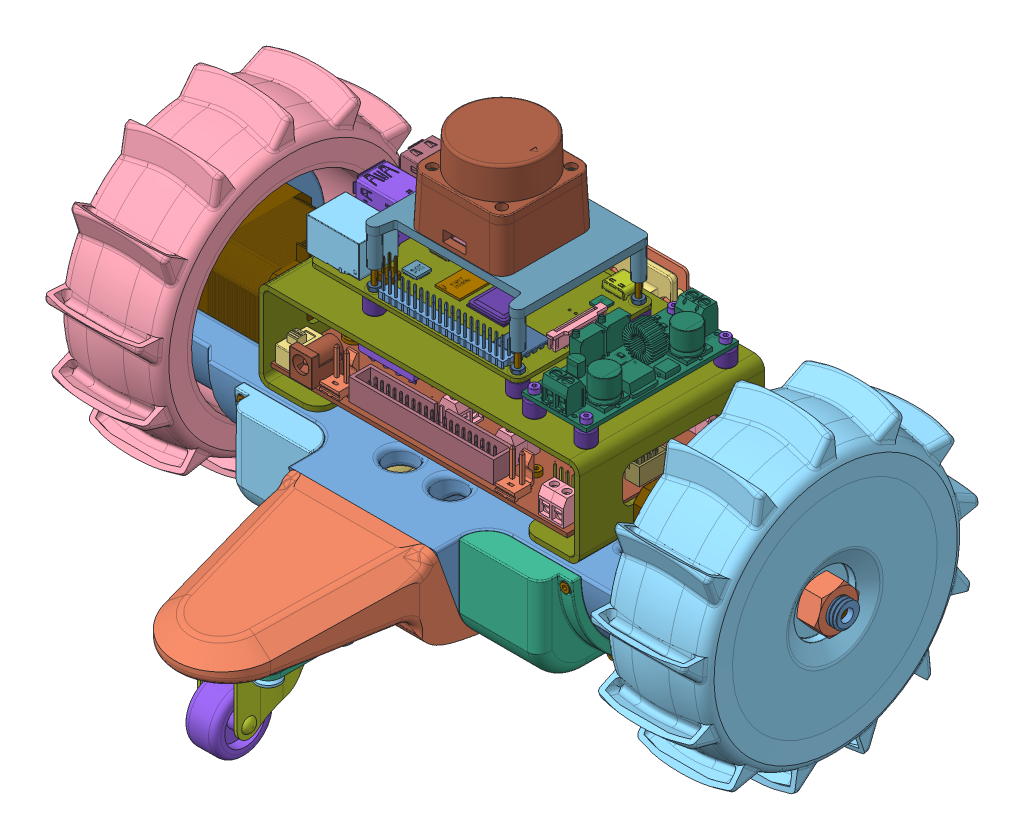
SolidWorks assembly RILeyV2_Assembly, configuration Default. Lengths in mm.
Overall size (273.39 192.08 229.11).
286 component instances, 95 part files, 157 mates.
Components (placement in the parent):
- MiddlepartV2-1: MiddlepartV2 [Default] at (252.5332 203.3689 525.8328) size (230.11 74.9 106.82)
- MiddlepartTailV2-1: MiddlepartTailV2 [Default] at (222.5332 176.6989 577.1871) size (60 37.63 93.1)
- 3_battery_pack-1: 3_battery_pack [Défaut] at (137.8855 170.9072 532.0524) x (0.340955 -0.94008 0) z (0.94008 0.340955 0) size (33.05 64.4 54.62)
  - Li-ion Battery-1: Li-ion Battery [Défaut] at (13.1472 -31.5804 64) size (18 64.02 18)
  - link2-1: link2 [Défaut] at (30.5553 32.4196 84.2976) x (-0.340955 0 -0.94008) z (0 1 0) size (44 5 0.2)
  - Li-ion Battery-2: Li-ion Battery [Défaut] at (19.2844 -31.5804 80.9214) x (0.492149 0 0.870511) z (-0.870511 0 0.492149) size (18 64.02 18)
  - Li-ion Battery-3: Li-ion Battery [Défaut] at (25.4216 -31.5804 97.8429) x (0.922234 0 -0.386631) z (0.386631 0 0.922234) size (18 64.02 18)
  - link2-2: link2 [Défaut] at (25.7705 -31.5804 71.1051) x (0.340955 0 0.94008) z (0 -1 0) size (44 5 0.2)
- 3_battery_pack-2: 3_battery_pack [Défaut] at (201.8855 170.9072 532.0524) x (0.340955 -0.94008 0) z (0.94008 0.340955 0) size (33.05 64.4 54.62)
  - Li-ion Battery-1: Li-ion Battery [Défaut] at (13.1472 -31.5804 64) size (18 64.02 18)
  - link2-1: link2 [Défaut] at (30.5553 32.4196 84.2976) x (-0.340955 0 -0.94008) z (0 1 0) size (44 5 0.2)
  - Li-ion Battery-2: Li-ion Battery [Défaut] at (19.2844 -31.5804 80.9214) x (0.492149 0 0.870511) z (-0.870511 0 0.492149) size (18 64.02 18)
  - Li-ion Battery-3: Li-ion Battery [Défaut] at (25.4216 -31.5804 97.8429) x (0.922234 0 -0.386631) z (0.386631 0 0.922234) size (18 64.02 18)
  - link2-2: link2 [Défaut] at (25.7705 -31.5804 71.1051) x (0.340955 0 0.94008) z (0 -1 0) size (44 5 0.2)
- BatteryCoverBackLeft-1: BatteryCoverBackLeft [Default] at (203.2832 163.3689 556.4) x (-1 0 0) z (0 0 -1) size (40.1 41.17 43.87)
- BatteryCoverBackRight-1: BatteryCoverBackRight [Default] at (301.7832 163.3689 556.4) x (-1 0 0) z (0 0 -1) size (40.1 41.17 43.86)
- BatteryCoverFront-1: BatteryCoverFront [Default] at (252.5332 164.3689 503.8328) size (137.1 39.19 32.19)
- Nema_17-17HS4401.step-1: Nema_17-17HS4401.step [Default] at (362.5332 203.3689 525.8328) x (0 1 0) z (1 0 0) size (47.8 42 64)
  - ConnectorPins.step-1: ConnectorPins.step [Default] at origin size (7 10.45 0.45)
    - SOLID.step-1: SOLID.step [Default] at origin size (7 0.45 0.45)
    - SOLID001.step-1: SOLID001.step [Default] at origin size (7 0.45 0.45)
    - SOLID002.step-1: SOLID002.step [Default] at origin size (7 0.45 0.45)
    - SOLID003.step-1: SOLID003.step [Default] at origin size (7 0.45 0.45)
    - SOLID004.step-1: SOLID004.step [Default] at origin size (7 0.45 0.45)
    - SOLID005.step-1: SOLID005.step [Default] at origin size (7 0.45 0.45)
  - Screws.step-1: Screws.step [Default] at origin size (36.6 36.6 32.35)
    - M3x30-Screw_001.step-1: M3x30-Screw_001.step [Default] at (15.5 15.5 -36.425) x (-1 0 0) z (0 0 -1) size (5.6 5.6 32.35)
    - M3x30-Screw_002.step-1: M3x30-Screw_002.step [Default] at (-15.5 15.5 -36.425) x (-1 0 0) z (0 0 -1) size (5.6 5.6 32.35)
    - M3x30-Screw_003.step-1: M3x30-Screw_003.step [Default] at (15.5 -15.5 -36.425) x (-1 0 0) z (0 0 -1) size (5.6 5.6 32.35)
    - M3x30-Screw_004.step-1: M3x30-Screw_004.step [Default] at (-15.5 -15.5 -36.425) x (-1 0 0) z (0 0 -1) size (5.6 5.6 32.35)
  - eBom-FreeParts-1: eBom-FreeParts [Default] at origin size (47.8 42 64)
- Nema_17-17HS4401.step-2: Nema_17-17HS4401.step [Default] at (142.5332 203.3689 525.8328) x (0 1 0) z (-1 0 0) size (47.8 42 64)
  - ConnectorPins.step-1: ConnectorPins.step [Default] at origin size (7 10.45 0.45)
    - SOLID.step-1: SOLID.step [Default] at origin size (7 0.45 0.45)
    - SOLID001.step-1: SOLID001.step [Default] at origin size (7 0.45 0.45)
    - SOLID002.step-1: SOLID002.step [Default] at origin size (7 0.45 0.45)
    - SOLID003.step-1: SOLID003.step [Default] at origin size (7 0.45 0.45)
    - SOLID004.step-1: SOLID004.step [Default] at origin size (7 0.45 0.45)
    - SOLID005.step-1: SOLID005.step [Default] at origin size (7 0.45 0.45)
  - Screws.step-1: Screws.step [Default] at origin size (36.6 36.6 32.35)
    - M3x30-Screw_001.step-1: M3x30-Screw_001.step [Default] at (15.5 15.5 -36.425) x (-1 0 0) z (0 0 -1) size (5.6 5.6 32.35)
    - M3x30-Screw_002.step-1: M3x30-Screw_002.step [Default] at (-15.5 15.5 -36.425) x (-1 0 0) z (0 0 -1) size (5.6 5.6 32.35)
    - M3x30-Screw_003.step-1: M3x30-Screw_003.step [Default] at (15.5 -15.5 -36.425) x (-1 0 0) z (0 0 -1) size (5.6 5.6 32.35)
    - M3x30-Screw_004.step-1: M3x30-Screw_004.step [Default] at (-15.5 -15.5 -36.425) x (-1 0 0) z (0 0 -1) size (5.6 5.6 32.35)
  - eBom-FreeParts-1: eBom-FreeParts [Default] at origin size (47.8 42 64)
- LeftWheelAssembly-1: LeftWheelAssembly [Default] at (238.5332 203.3689 525.8328) size (46.89 175.5 175.66)
  - HexBolt_modified-1: HexBolt_modified [Default] at (-101 0 0) x (0 0 1) z (-1 0 0) size (19.63 17 21.55)
  - hex nut style 1 gradeab_din-1: hex nut style 1 gradeab_din [Hexagon Nut ISO 4032 - M10 - D - S] at (-118.4 0 0) x (0 0 1) z (-1 0 0) size (16 18.48 8.4)
  - socket set screw cup point_din-1: socket set screw cup point_din [DIN 916 - M3 x 5-S] at (-104 7.5 0) x (0 -1 0) z (-0.467009 0 0.884252) size (5 3 3)
  - ReelyBuggyWheel_Left-2: ReelyBuggyWheel_Left [Default] at (-96.5 0 0) x (0 -0.851174 0.524883) z (-1 0 0) size (127.36 127.83 41.68)
- RightWheelAssembly-1: RightWheelAssembly [Default] at (335.8173 229.3376 519.6115) x (-0.999996 0.002302 0.001897) z (-0.002983 -0.771739 -0.635933) size (47.18 164.08 164.48)
  - hex nut style 1 gradeab_din-2: hex nut style 1 gradeab_din [Hexagon Nut ISO 4032 - M10 - D - S] at (-40.7637 -21.3156 15.9632) x (0.002628 0.473226 -0.880937) z (0.999996 0 0.002983) size (16 18.48 8.4)
  - ReelyBuggyWheel_Right-1: ReelyBuggyWheel_Right [Default] at (-27.2638 -21.3156 16.0035) x (0.001045 0.936608 -0.350379) z (-0.999996 0 -0.002983) size (127.36 127.83 41.68)
  - socket set screw cup point_din-1: socket set screw cup point_din [DIN 916 - M3 x 5-S] at (-34.7467 -16.6097 10.2703) x (-0.002302 -0.635936 0.771739) z (-0.466048 0.683487 0.561824) size (5 3 3)
  - HexBolt_modified-1: HexBolt_modified [Default] at (-31.7638 -21.3156 15.9901) x (-0.001897 0.771742 0.635933) z (-0.999996 0 -0.002983) size (19.63 17 21.55)
- SwivelWheel-1: SwivelWheel [Default] at (228.6024 159.2147 634.0467) x (0 0 -1) z (1 0 0) size (49.24 37.2 40)
  - SwivelWheelBase-1: SwivelWheelBase [Default] at (-10.4964 21.1542 43.9308) size (40 5 40)
  - SwivelWheelMid-1: SwivelWheelMid [Default] at (9.5036 -14.3458 23.9308) x (0.99994 0 -0.010997) z (0.010997 0 0.99994) size (30.88 25.42 20)
  - SwivelWheelWheel-1: SwivelWheelWheel [Default] at (-6.5669 -0.8742 17.6072) x (-0.010997 0 -0.99994) z (0.05546 0.998461 -0.00061) size (13 25 25)
- RILey_PCB_V2-1: RILey_PCB_V2 [Default] at (282.1383 155.4598 627.7401) x (-1 0 0) z (0 0 -1) size (120 36.8 77.07)
  - RILey-PCB_V2.0.step-1: RILey-PCB_V2.0.step [Default] at (-30.3949 55.9091 134.4073) x (1 0 0) z (0 1 0) size (120 77.07 36.8)
    - Packages.step-1: Packages.step [Default] at origin size (117.53 77.07 36.8)
      - CAPPRD250W50D655H1250.step-1: CAPPRD250W50D655H1250.step [Default] at (10.16 48.26 1.57) x (-1 0 0) z (0 0 1) size (7.62 7.6 12.92)
        - Model.step-1: Model.step [Default] at (1.2482 -0.0007 0.1237) size (7.62 7.6 12.92)
      - CAPPRD250W50D655H1250_1.step-1: CAPPRD250W50D655H1250_1.step [Default] at (110.49 44.45 1.57) size (7.62 7.6 12.92)
        - Model.step-1: Model.step [Default] at (1.2482 -0.0007 0.1237) size (7.62 7.6 12.92)
      - ELECTROLYTIC_CAPACITOR.step-1: ELECTROLYTIC_CAPACITOR.step [Default] at (20.32 5.08 1.57) size (8.02 8 21.92)
        - Model (1).step-1: Model (1).step [Default] at origin size (8.02 8 21.92)
      - 733980-62.step-1: 733980-62.step [Default] at (106.68 66.04 1.57) x (-1 0 0) z (0 0 1) size (9.55 14.2 15)
        - DS-210 v1.step-1: DS-210 v1.step [Default] at (-0.0014 -5.2814 0) x (-1 0 0) z (0 0 1) size (9.55 14.2 15)
      - B4B-XH-A_LF__SN_.step-1: B4B-XH-A_LF__SN_.step [Default] at (5.08 29.21 1.57) x (0 1 0) z (0 0 1) size (12.4 5.75 10.45)
        - JST XH 4 B4B-XH-A v1.step-1: JST XH 4 B4B-XH-A v1.step [Default] at (3.6633 0.5127 0.0202) x (1 0 0) z (0 -1 0) size (12.4 10.45 5.75)
      - B4B-XH-A_LF__SN_.step-2: B4B-XH-A_LF__SN_.step [Default] at (115.57 34.29 1.57) x (0 -1 0) z (0 0 1) size (12.4 5.75 10.45)
        - JST XH 4 B4B-XH-A v1.step-1: JST XH 4 B4B-XH-A v1.step [Default] at (3.6633 0.5127 0.0202) x (1 0 0) z (0 -1 0) size (12.4 10.45 5.75)
      - MC-254-40-00-ST-DIP.step-1: MC-254-40-00-ST-DIP.step [Default] at (61.214 63.5 1.57) size (58.67 8.85 11.85)
        - MC-254-40-00-ST-DIP v1.step-1: MC-254-40-00-ST-DIP v1.step [Default] at (-24.13 -1.27 0) size (58.67 8.85 11.85)
          - Model (2).step-1: Model (2).step [Default] at (0 2.54 0) size (58.67 8.85 11.85)
      - TSOP6_SOT457.step-1: TSOP6_SOT457.step [Default] at (17.78 48.26 0) x (-1 0 0) z (0 0 -1) size (3 3.1 1.1)
        - Model (3).step-1: Model (3).step [Default] at origin size (3 3.1 1.1)
      - ZENER-TH.step-1: ZENER-TH.step [Default] at (75.565 14.605 1.57) x (0 1 0) z (0 0 1) size (8.22 2 4.02)
        - Model (4).step-1: Model (4).step [Default] x (-1 0 0) z (0 0 1) size (8.22 2 4.02)
      - 1812L300MR.step-1: 1812L300MR.step [Default] at (71.0315 17.78 0) x (0 -1 0) z (0 0 -1) size (4.73 3.41 1)
        - Model (5).step-1: Model (5).step [Default] at origin size (4.73 3.41 1)
      - 2920L400_15MR.step-1: 2920L400_15MR.step [Default] at (109.22 52.07 0) x (1 0 0) z (0 0 -1) size (7.98 5.44 1.6)
        - Model (6).step-1: Model (6).step [Default] at origin size (7.98 5.44 1.6)
      - MA04-1W.step-1: MA04-1W.step [Default] at (42.0116 3.8608 1.57) x (-1 0 0) z (0 0 1) size (10.16 9.88 5.54)
        - Model (7).step-1: Model (7).step [Default] at (3.81 -0.002 0) x (-1 0 0) z (0 0 1) size (10.16 9.89 5.54)
      - MA15-1W.step-1: MA15-1W.step [Default] at (76.2 3.81 1.57) x (-1 0 0) z (0 0 1) size (38.1 9.89 5.54)
        - Model (8).step-1: Model (8).step [Default] at (17.78 0 0) x (-1 0 0) z (0 0 1) size (38.1 9.89 5.54)
      - KK41791-4020_2-PIN.step-1: KK41791-4020_2-PIN.step [Default] at (96.52 64.77 1.57) x (-1 0 0) z (0 0 1) size (7.77 10.01 17.02)
        - Molex-kk-396 v2.step-1: Molex-kk-396 v2.step [Default] at (0.0973 -2.0339 0.4801) x (1 0 0) z (0 -1 0) size (7.77 17.02 10.01)
          - 1.step-1: 1.step [Default] at (-0.1266 1.3496 -0.3443) size (7.77 17.02 10.01)
      - KK41791-4020_2-PIN_1.step-1: KK41791-4020_2-PIN_1.step [Default] at (25.4 64.77 1.57) x (-1 0 0) z (0 0 1) size (7.77 10.01 17.02)
        - Molex-kk-396 v2_1.step-1: Molex-kk-396 v2_1.step [Default] at (0.0973 -2.0339 0.4801) x (1 0 0) z (0 -1 0) size (7.77 17.02 10.01)
          - 1.step-1: 1.step [Default] at (-0.1266 1.3496 -0.3443) size (7.77 17.02 10.01)
      - 1000-SERIES(SPDT).step-1: 1000-SERIES(SPDT).step [Default] at (115.6208 62.7634 1.57) size (7.2 13 13.1)
        - SS-12M11G3 v2.step-1: SS-12M11G3 v2.step [Default] at origin size (7.2 13 13.1)
      - W237-102.step-1: W237-102.step [Default] at (7.5692 66.3194 1.57) size (10.66 8 14)
        - Schraubklemme_Blau_300V_16A_2P v1.step-1: Schraubklemme_Blau_300V_16A_2P v1.step [Default] at (-0.2451 0.529 2.8414) x (0 1 0) z (0 0 1) size (8 10.66 14)
          - Schraubklemme_Blau_300V_16A.step-1: Schraubklemme_Blau_300V_16A.step [Default] at (2.2082 -5.3326 -3) size (8 5.58 14)
          - Schraubklemme_Blau_300V_16A.step-2: Schraubklemme_Blau_300V_16A.step [Default] at (2.2082 -0.2526 -3) size (8 5.58 14)
      - W237-102_1.step-1: W237-102_1.step [Default] at (8.89 3.81 1.57) x (-1 0 0) z (0 0 1) size (10.66 8 14)
        - Schraubklemme_Blau_300V_16A_2P v1_1.step-1: Schraubklemme_Blau_300V_16A_2P v1_1.step [Default] at (-0.2451 0.529 2.8414) x (0 1 0) z (0 0 1) size (8 10.66 14)
          - Schraubklemme_Blau_300V_16A.step-1: Schraubklemme_Blau_300V_16A.step [Default] at (2.2082 -5.3326 -3) size (8 5.58 14)
          - Schraubklemme_Blau_300V_16A.step-2: Schraubklemme_Blau_300V_16A.step [Default] at (2.2082 -0.2526 -3) size (8 5.58 14)
      - W237-102_2.step-1: W237-102_2.step [Default] at (59.5884 52.07 1.57) x (0 1 0) z (0 0 1) size (10.66 8 14)
        - Schraubklemme_Blau_300V_16A_2P v1_2.step-1: Schraubklemme_Blau_300V_16A_2P v1_2.step [Default] at (-0.2451 0.529 2.8414) x (0 1 0) z (0 0 1) size (8 10.66 14)
          - Schraubklemme_Blau_300V_16A.step-1: Schraubklemme_Blau_300V_16A.step [Default] at (2.2082 -5.3326 -3) size (8 5.58 14)
          - Schraubklemme_Blau_300V_16A.step-2: Schraubklemme_Blau_300V_16A.step [Default] at (2.2082 -0.2526 -3) size (8 5.58 14)
      - W237-102_3.step-1: W237-102_3.step [Default] at (39.37 52.07 1.57) x (0 -1 0) z (0 0 1) size (10.66 8 14)
        - Schraubklemme_Blau_300V_16A_2P v1_3.step-1: Schraubklemme_Blau_300V_16A_2P v1_3.step [Default] at (-0.2451 0.529 2.8414) x (0 1 0) z (0 0 1) size (8 10.66 14)
          - Schraubklemme_Blau_300V_16A.step-1: Schraubklemme_Blau_300V_16A.step [Default] at (2.2082 -5.3326 -3) size (8 5.58 14)
          - Schraubklemme_Blau_300V_16A.step-2: Schraubklemme_Blau_300V_16A.step [Default] at (2.2082 -0.2526 -3) size (8 5.58 14)
      - FE04-1.step-1: FE04-1.step [Default] at (52.2732 15.6464 1.57) x (-1 0 0) z (0 0 1) size (10.16 2.5 11.3)
      - FE10-1.step-1: FE10-1.step [Default] at (66.04 19.0691 1.57) x (0 -1 0) z (0 0 1) size (25.9 2.5 11.3)
      - MA05-1_S.step-1: MA05-1_S.step [Default] at (13.97 55.88 1.57) x (-1 0 0) z (0 0 1) size (13.2 2.5 11)
      - DIODE-BRIDGE.step-1: DIODE-BRIDGE.step [Default] at (92.71 48.26 1.57) size (22.51 3.56 36.8)
      - FE08-1.step-1: FE08-1.step [Default] at (25.4 33.02 1.57) x (0 1 0) z (0 0 1) size (20.82 2.5 11.3)
      - FE08-1.step-2: FE08-1.step [Default] at (12.7 33.02 1.57) x (0 1 0) z (0 0 1) size (20.82 2.5 11.3)
      - FE08-1.step-3: FE08-1.step [Default] at (95.25 30.48 1.57) x (0 -1 0) z (0 0 1) size (20.82 2.5 11.3)
      - FE08-1.step-4: FE08-1.step [Default] at (107.95 30.48 1.57) x (0 -1 0) z (0 0 1) size (20.82 2.5 11.3)
      - MA04-1_S.step-1: MA04-1_S.step [Default] at (99.06 7.62 1.57) x (0 -1 0) z (0 0 1) size (10.66 2.5 11)
      - MA04-1_S.step-2: MA04-1_S.step [Default] at (104.14 7.62 1.57) x (0 -1 0) z (0 0 1) size (10.66 2.5 11)
      - MA04-1_S.step-3: MA04-1_S.step [Default] at (110.49 7.62 1.57) x (0 -1 0) z (0 0 1) size (10.66 2.5 11)
      - MA04-1_S.step-4: MA04-1_S.step [Default] at (115.57 7.62 1.57) x (0 -1 0) z (0 0 1) size (10.66 2.5 11)
    - Board.step-1: Board.step [Default] at origin size (120 70 1.57)
  - DRV 8825 With Headers Assem-1: DRV 8825 With Headers Assem [Default] at (-1.0467 51.8574 109.5035) x (0 0 -1) z (0 1 0) size (21 15 10.9)
    - PCB-1: PCB [Default] at (8.1162 10.2982 16.4218) size (21 15 1.8)
    - SMD Pot-1: SMD Pot [Default] at (-0.2134 7.4613 18.0218) x (0 -1 0) z (0 0 1) size (3 3 1.3)
    - 0603 Resistor-1: 0603 Resistor [Default] at (-1.0068 10.8561 18.0218) size (1.5 0.8 0.5)
    - 0603 Resistor-2: 0603 Resistor [Default] at (-1.0286 12.2306 18.0218) size (1.5 0.8 0.5)
    - 0805 Capacitor-1: 0805 Capacitor [Default] at (-0.8941 14.0417 18.0218) size (2 1.25 1.25)
    - 0402 Resistor-1: 0402 Resistor [Default] at (16.8896 6.6863 18.0218) x (0 -1 0) z (0 0 1) size (1 0.68 0.66)
    - 0402 Resistor-2: 0402 Resistor [Default] at (16.8896 10.308 18.0218) x (0 -1 0) z (0 0 1) size (1 0.68 0.66)
    - 0402 Resistor-3: 0402 Resistor [Default] at (16.8896 13.6408 18.0218) x (0 -1 0) z (0 0 1) size (1 0.68 0.66)
    - 0402 Resistor-4: 0402 Resistor [Default] at (6.8882 6.5987 18.0218) x (0 -1 0) z (0 0 1) size (1 0.68 0.66)
    - 0402 Resistor-5: 0402 Resistor [Default] at (5.9719 6.5987 18.0218) x (0 -1 0) z (0 0 1) size (1 0.68 0.66)
    - 0402 Resistor-6: 0402 Resistor [Default] at (5.456 14.3274 18.0218) size (1 0.68 0.66)
    - 0402 Resistor-7: 0402 Resistor [Default] at (5.456 13.4855 18.0218) size (1 0.68 0.66)
    - DRV8825 IC-1: DRV8825 IC [Default] at (11.7347 10.2312 18.0218) x (0 -1 0) z (0 0 1) size (9.6 6.2 1.2)
    - 8 pin Header-1: 8 pin Header [Default] at (8.1162 16.2982 13.9218) size (21 2.5 10.5)
    - 8 pin Header-2: 8 pin Header [Default] at (8.1162 4.2982 13.9218) size (21 2.5 10.5)
  - DRV 8825 With Headers Assem-2: DRV 8825 With Headers Assem [Default] at (60.9069 51.8574 95.811) x (0 0 1) z (0 1 0) size (21 15 10.9)
    - PCB-1: PCB [Default] at (8.1162 10.2982 16.4218) size (21 15 1.8)
    - SMD Pot-1: SMD Pot [Default] at (-0.2134 7.4613 18.0218) x (0 -1 0) z (0 0 1) size (3 3 1.3)
    - 0603 Resistor-1: 0603 Resistor [Default] at (-1.0068 10.8561 18.0218) size (1.5 0.8 0.5)
    - 0603 Resistor-2: 0603 Resistor [Default] at (-1.0286 12.2306 18.0218) size (1.5 0.8 0.5)
    - 0805 Capacitor-1: 0805 Capacitor [Default] at (-0.8941 14.0417 18.0218) size (2 1.25 1.25)
    - 0402 Resistor-1: 0402 Resistor [Default] at (16.8896 6.6863 18.0218) x (0 -1 0) z (0 0 1) size (1 0.68 0.66)
    - 0402 Resistor-2: 0402 Resistor [Default] at (16.8896 10.308 18.0218) x (0 -1 0) z (0 0 1) size (1 0.68 0.66)
    - 0402 Resistor-3: 0402 Resistor [Default] at (16.8896 13.6408 18.0218) x (0 -1 0) z (0 0 1) size (1 0.68 0.66)
    - 0402 Resistor-4: 0402 Resistor [Default] at (6.8882 6.5987 18.0218) x (0 -1 0) z (0 0 1) size (1 0.68 0.66)
    - 0402 Resistor-5: 0402 Resistor [Default] at (5.9719 6.5987 18.0218) x (0 -1 0) z (0 0 1) size (1 0.68 0.66)
    - 0402 Resistor-6: 0402 Resistor [Default] at (5.456 14.3274 18.0218) size (1 0.68 0.66)
    - 0402 Resistor-7: 0402 Resistor [Default] at (5.456 13.4855 18.0218) size (1 0.68 0.66)
    - DRV8825 IC-1: DRV8825 IC [Default] at (11.7347 10.2312 18.0218) x (0 -1 0) z (0 0 1) size (9.6 6.2 1.2)
    - 8 pin Header-1: 8 pin Header [Default] at (8.1162 16.2982 13.9218) size (21 2.5 10.5)
    - 8 pin Header-2: 8 pin Header [Default] at (8.1162 4.2982 13.9218) size (21 2.5 10.5)
  - MPU9250.STEP-1: MPU9250.STEP [Default] at (68.1451 69.3424 118.518) x (0 0 1) z (-1 0 0) size (26 3.91 16)
    - PCB.STEP-1: PCB.STEP [Default] at (-2.9998 1.0768 26) size (26 2.2 16)
    - C2.STEP-1: C2.STEP [Default] at (-2.4989 2.0768 21) x (0 0 -1) z (1 0 0) size (2 1.81 5.01)
    - MP92.STEP-1: MP92.STEP [Default] at (-2.9998 1.0968 25.5) x (0 0 -1) z (1 0 0) size (3.29 1.01 3.29)
    - C1_Predeterminado_Como mecanizada_.STEP-1: C1_Predeterminado_Como mecanizada_.STEP [Default] at (2.1384 1.0968 23.0905) x (0 0 1) z (-1 0 0) size (2.2 0.83 0.9)
    - C1_Predeterminado_Como mecanizada_.STEP-2: C1_Predeterminado_Como mecanizada_.STEP [Default] at (0.9102 1.0968 27.1044) x (0 0 1) z (-1 0 0) size (2.2 0.83 0.9)
    - C1_Predeterminado_Como mecanizada_.STEP-3: C1_Predeterminado_Como mecanizada_.STEP [Default] at (0.9102 1.0968 23.0905) x (0 0 1) z (-1 0 0) size (2.2 0.83 0.9)
    - C1_Predeterminado_Como mecanizada_.STEP-4: C1_Predeterminado_Como mecanizada_.STEP [Default] at (-8.3098 1.0968 23.0905) x (0 0 1) z (-1 0 0) size (2.2 0.83 0.9)
    - C1_Predeterminado_Como mecanizada_.STEP-5: C1_Predeterminado_Como mecanizada_.STEP [Default] at (-9.7098 1.0968 27.1044) x (0 0 1) z (-1 0 0) size (2.2 0.83 0.9)
    - R1.STEP-1: R1.STEP [Default] at (3.5484 1.1168 27.2144) x (0 0 -1) z (1 0 0) size (2.2 0.47 0.9)
    - R1.STEP-2: R1.STEP [Default] at (2.1484 1.1168 27.2144) x (0 0 -1) z (1 0 0) size (2.2 0.47 0.9)
    - R1.STEP-3: R1.STEP [Default] at (-6.8998 1.1168 23.2005) x (0 0 -1) z (1 0 0) size (2.2 0.47 0.9)
    - R1.STEP-4: R1.STEP [Default] at (-8.2998 1.1168 27.2144) x (0 0 -1) z (1 0 0) size (2.2 0.47 0.9)
    - R1.STEP-5: R1.STEP [Default] at (-6.8998 1.1168 27.2144) x (0 0 -1) z (1 0 0) size (2.2 0.47 0.9)
    - V1.STEP-1: V1.STEP [Default] at (-13.0785 1.5868 25.9) size (2.9 0.96 3.2)
  - PinHeader10row-1: PinHeader10row [Default] at (36.9151 68.3191 125.4982) x (0 0 1) z (1 0 0) size (25.4 11.54 2.54)
- 3rdFloorAssembly-1: 3rdFloorAssembly [Default] at (252.5332 203.3689 525.8328) size (130 100.19 75)
  - socket head cap screw 4762_din-1: socket head cap screw 4762_din [EN ISO 4762 M2 x 12 - 12S] at (37.5 45.65 -28.25) x (0 -1 0) z (0 0 1) size (14 3.8 3.8)
  - socket head cap screw 4762_din-2: socket head cap screw 4762_din [EN ISO 4762 M2 x 12 - 12S] at (58.5 45.65 -28.25) x (0 -1 0) z (0 0 1) size (14 3.8 3.8)
  - socket head cap screw 4762_din-3: socket head cap screw 4762_din [EN ISO 4762 M2 x 12 - 12S] at (58.5 45.65 28.25) x (0 -1 0) z (0 0 1) size (14 3.8 3.8)
  - socket head cap screw 4762_din-4: socket head cap screw 4762_din [EN ISO 4762 M2 x 12 - 12S] at (37.5 45.65 28.25) x (0 -1 0) z (0 0 1) size (14 3.8 3.8)
  - socket head cap screw_iso-1: socket head cap screw_iso [ISO 4762 M2 x 20 - 20C] at (-31 32 -24.5) x (0 1 0) z (0 0 1) size (22 3.8 3.8)
  - socket head cap screw_iso-2: socket head cap screw_iso [ISO 4762 M2 x 20 - 20C] at (-31 32 24.5) x (0 1 0) z (0 0 1) size (22 3.8 3.8)
  - socket head cap screw_iso-3: socket head cap screw_iso [ISO 4762 M2 x 20 - 20C] at (27 32 -24.5) x (0 1 0) z (0 0 1) size (22 3.8 3.8)
  - socket head cap screw_iso-4: socket head cap screw_iso [ISO 4762 M2 x 20 - 20C] at (27 32 24.5) x (0 1 0) z (0 0 1) size (22 3.8 3.8)
  - hex nut style 1 gradeab_iso-1: hex nut style 1 gradeab_iso [ISO - 4032 - M2 - W - C] at (-31 45.19 -24.5) x (1 0 0) z (0 1 0) size (4 4.62 1.6)
  - hex nut style 1 gradeab_iso-2: hex nut style 1 gradeab_iso [ISO - 4032 - M2 - W - C] at (27 45.19 -24.5) x (1 0 0) z (0 1 0) size (4 4.62 1.6)
  - hex nut style 1 gradeab_iso-3: hex nut style 1 gradeab_iso [ISO - 4032 - M2 - W - C] at (-31 45.19 24.5) x (1 0 0) z (0 1 0) size (4 4.62 1.6)
  - hex nut style 1 gradeab_iso-4: hex nut style 1 gradeab_iso [ISO - 4032 - M2 - W - C] at (27 45.19 24.5) x (1 0 0) z (0 1 0) size (4 4.62 1.6)
  - hex nut style 1 gradeab_iso-5: hex nut style 1 gradeab_iso [ISO - 4032 - M2 - W - C] at (58.5 32.4 -28.25) x (1 0 0) z (0 -1 0) size (4 4.62 1.6)
  - hex nut style 1 gradeab_iso-6: hex nut style 1 gradeab_iso [ISO - 4032 - M2 - W - C] at (37.5 32.4 -28.25) x (1 0 0) z (0 -1 0) size (4 4.62 1.6)
  - hex nut style 1 gradeab_iso-7: hex nut style 1 gradeab_iso [ISO - 4032 - M2 - W - C] at (37.5 32.4 28.25) x (1 0 0) z (0 -1 0) size (4 4.62 1.6)
  - hex nut style 1 gradeab_iso-8: hex nut style 1 gradeab_iso [ISO - 4032 - M2 - W - C] at (58.5 32.4 28.25) x (1 0 0) z (0 -1 0) size (4 4.62 1.6)
  - LD06_Assembly-1: LD06_Assembly [Default] at (-60.828 42.1202 31.9351) x (0 0 -1) z (1 0 0) size (54 48.5 63)
    - LD06_LiDAR-1: LD06_LiDAR [Default] at (15.6414 21.3154 28.1688) size (38.59 33.3 38.59)
      - LD06_LiDAR-1: LD06_LiDAR [Default] at (16.3187 3.4544 28.6342) size (38.59 33.3 38.59)
      - JIS_B1111_M2x6.step-1: JIS_B1111_M2x6.step [Default] at (30.4187 21.1806 42.7342) x (1 0 0) z (0 1 0) size (3.5 3.5 7.3)
      - JIS_B1111_M2x6.step-2: JIS_B1111_M2x6.step [Default] at (2.2187 21.1806 14.5342) x (1 0 0) z (0 1 0) size (3.5 3.5 7.3)
      - jst-1.5mm-4P.step-1: jst-1.5mm-4P.step [Default] at (4.0237 7.1794 28.6342) x (0 0 -1) z (0 1 0) size (7.5 7.2 3.5)
    - LD06_PiBracket-1: LD06_PiBracket [Default] at (31.9351 21.5698 58.828) x (0 0 1) z (-1 0 0) size (63 27 54)
  - dc-dc-5a-cc-merged-1: dc-dc-5a-cc-merged [Default] at (48 43.6 0) x (0 0 -1) z (1 0 0) size (61.7 17.87 26.2)
  - Raspberry Pi 4 Model B-1: Raspberry Pi 4 Model B [Default] at (-12 42.8 0) x (-1 0 0) z (0 0 -1) size (88.99 19.9 58.4)
    - PCB, RPi4ModelB-1: PCB, RPi4ModelB [Default] at origin size (85 1.6 56)
    - Broadcom BCM2711B0 CPU, RPi4ModelB-1: Broadcom BCM2711B0 CPU, RPi4ModelB [Default] at (-13.25 0.8 -4.5) size (15 2.3 15)
    - 2.54 mm DUPONT MALE PIN HEADER, POE, 2X2, RPi4ModelB-1: 2.54 mm DUPONT MALE PIN HEADER, POE, 2X2, RPi4ModelB [Default] at (19 0.8 -18.5) size (5.08 11.3 5.08)
    - 2.54 mm DUPONT MALE PIN HEADER, IO, 2X20, RPi4ModelB-1: 2.54 mm DUPONT MALE PIN HEADER, IO, 2X20, RPi4ModelB [Default] at (-10 0.8 -24.5) size (50.8 11.3 5.08)
    - Camera Connector, RPi4ModelB-1: Camera Connector, RPi4ModelB [Default] at (4 0.8 16.5) x (0 0 -1) z (1 0 0) size (22.4 5.68 5.07)
    - Microphone Plug, RPi4ModelB-1: Microphone Plug, RPi4ModelB [Default] at (11.5 0.8 21.65) size (7.23 7.55 15)
    - Display Connector, RPi4ModelB-1: Display Connector, RPi4ModelB [Default] at (-38.5 0.8 0) x (0 0 1) z (-1 0 0) size (22.4 5.68 5.07)
    - Gigabit Ethernet Port, RPi4ModelB-1: Gigabit Ethernet Port, RPi4ModelB [Default] at (45.5 7.55 -17.75) x (0 0 -1) z (1 0 0) size (16.2 17.24 21.64)
    - Female Micro HDMI Connector, RPi4ModelB-2: Female Micro HDMI Connector, RPi4ModelB [Default] at (-3 0.8 27.3875) size (6.5 3.51 7.5)
    - Female Micro HDMI Connector, RPi4ModelB-3: Female Micro HDMI Connector, RPi4ModelB [Default] at (-16.5 0.8 27.3875) size (6.5 3.51 7.5)
    - Female USB Type C Connector, RPi4ModelB-1: Female USB Type C Connector, RPi4ModelB [Default] at (-31.3 0.8 26.5419) size (8.94 3.96 7.9)
    - 2X USB3.0 PORTS, RPi4ModelB-2: 2X USB3.0 PORTS, RPi4ModelB [Default] at (37.07 0.8 1) size (17.47 19.41 15.68)
    - 91D77 D9WHV 778K, 4 GB LPDDR4 SDRAM, RPi4ModelB-1: 91D77 D9WHV 778K, 4 GB LPDDR4 SDRAM, RPi4ModelB [Default] at (2.25 0.8 -4.5) size (10 0.8 14.5)
    - Cypress CYW43455 Wireless Module Cover, RPi4ModelB-1: Cypress CYW43455 Wireless Module Cover, RPi4ModelB [Default] at (-30.5 0.8 -14.5) size (11 1.6 13)
    - SD Card Slot, RPi4ModelB-1: SD Card Slot, RPi4ModelB [Default] at (-35.3 -0.8 0) x (0 0 -1) z (-1 0 0) size (11.95 1.45 11.4)
    - VIA VL805 PCIe USB 3.0 controller, RPi4ModelB-1: VIA VL805 PCIe USB 3.0 controller, RPi4ModelB [Default] at (17.5 0.8 4) size (8.8 0.8 8.8)
    - 2X USB2.0 PORTS, RPi4ModelB-1: 2X USB2.0 PORTS, RPi4ModelB [Default] at (37.065 0.65 19) size (17.87 19.16 15.33)
    - Broadcom BCM54213PE Gigabit Ethernet Transceiver, RPi4ModelB-1: Broadcom BCM54213PE Gigabit Ethernet Transceiver, RPi4ModelB [Default] at (16.5 0.8 -10) size (6.8 1 6.8)
    - MxL7704 Universal PMIC, RPi4ModelB-1: MxL7704 Universal PMIC, RPi4ModelB [Default] at (-32.5 0.8 16) size (5.4 0.8 5.4)
  - 3rdFloor_Sheetmetal-1: 3rdFloor_Sheetmetal [Default] at (0 36 0) size (130 36 75)
  - Spacer-1: Spacer [Default] at (37.5 36 -28.25) x (-0.470741 0 0.882271) z (-0.882271 0 -0.470741) size (7 6 7)
  - Spacer-2: Spacer [Default] at (58.5 36 -28.25) x (0.784801 0 0.619748) z (-0.619748 0 0.784801) size (7 6 7)
  - Spacer-3: Spacer [Default] at (-31 36 24.5) size (7 6 7)
  - Spacer-4: Spacer [Default] at (37.5 36 28.25) x (0.517299 0 -0.855805) z (0.855805 0 0.517299) size (7 6 7)
  - Spacer-5: Spacer [Default] at (58.5 36 28.25) size (7 6 7)
  - Spacer-6: Spacer [Default] at (27 36.3 -24.5) x (-0.705828 0 0.708384) z (-0.708384 0 -0.705828) size (7 6 7)
  - Spacer-7: Spacer [Default] at (27 36 24.5) x (0.999844 0 -0.017672) z (0.017672 0 0.999844) size (7 6 7)
  - Spacer-8: Spacer [Default] at (-31 36 -24.5) x (-0.657111 0 -0.753794) z (0.753794 0 -0.657111) size (7 6 7)
- TimeOfFlightAssembly-1: TimeOfFlightAssembly [Default] at (252.5332 242.1908 499.8675) x (-1 0 0) z (0 0.924225 0.381849) size (28 16.66 17.76)
  - TimeOfFlightMount-1: TimeOfFlightMount [Default] at (0 -3.6203 -48.3357) x (-1 0 0) z (0 -0.87922 0.476417) size (28 12 8.25)
  - VL53l1X-1: VL53l1X [Varsayılan] at (0 -6.8924 -51.2259) x (-1 0 0) z (0 -0.87922 0.476417) size (25 4 10.5)
  - hex nut style 1 gradeab_iso-1: hex nut style 1 gradeab_iso [ISO - 4032 - M3 - W - N] at (-10 -3.7957 -45.511) x (1 0 0) z (0 0.476417 0.87922) size (5.5 6.35 2.4)
  - hex nut style 1 gradeab_iso-2: hex nut style 1 gradeab_iso [ISO - 4032 - M3 - W - N] at (10 -3.7957 -45.511) x (-0.997793 -0.058376 0.031632) z (0 0.476417 0.87922) size (5.5 6.35 2.4)
  - socket head cap screw_iso-1: socket head cap screw_iso [ISO 4762 M3 x 8 - 8C] at (-10 -9.0839 -55.2703) x (0 0.476417 0.87922) z (-0.87922 -0.418875 0.226973) size (11 5.5 5.5)
  - socket head cap screw_iso-2: socket head cap screw_iso [ISO 4762 M3 x 8 - 8C] at (10 -9.0839 -55.2703) x (0 0.476417 0.87922) z (-0.87922 -0.418875 0.226973) size (11 5.5 5.5)
- CameraAssembly-1: CameraAssembly [Default] at (252.5332 200.2861 525.4104) x (1 0 0) z (0 -0.083651 0.996495) size (25.31 32.26 33.3)
  - Cam V2.1 v1.step-1: Cam V2.1 v1.step [Default] at (0 16.3492 -59.3807) x (0 -0.098914 -0.995096) z (-1 0 0) size (6.45 24 25)
  - CameraMount-1: CameraMount [Default] at (-12.5 4.7048 -55.2085) x (1 0 0) z (0 0.098914 0.995096) size (25.31 30.03 24.03)
  - socket head cap screw_din-1: socket head cap screw_din [DIN 912 M2 x 10 --- 10S] at (-10.5 18.5402 -62.6133) x (0 0.098914 0.995096) z (-0.995096 -0.098429 0.009784) size (12 3.8 3.8)
  - socket head cap screw_din-2: socket head cap screw_din [DIN 912 M2 x 10 --- 10S] at (-10.5 6.1015 -61.3769) x (0 0.098914 0.995096) z (-0.995096 -0.098429 0.009784) size (12 3.8 3.8)
  - socket head cap screw_din-3: socket head cap screw_din [DIN 912 M2 x 10 --- 10S] at (10.5 6.1015 -61.3769) x (0 0.098914 0.995096) z (-0.995096 -0.098429 0.009784) size (12 3.8 3.8)
  - socket head cap screw_din-4: socket head cap screw_din [DIN 912 M2 x 10 --- 10S] at (10.5 18.5402 -62.6133) x (0 0.098914 0.995096) z (-0.995096 -0.098429 0.009784) size (12 3.8 3.8)
  - hex nut style 1 gradeab_din-1: hex nut style 1 gradeab_din [Hexagon Nut ISO 4032 - M2 - D - S] at (-10.5 19.5887 -52.0653) x (1 0 0) z (0 0.098914 0.995096) size (4 4.62 1.6)
  - hex nut style 1 gradeab_din-2: hex nut style 1 gradeab_din [Hexagon Nut ISO 4032 - M2 - D - S] at (10.5 19.5887 -52.0653) x (1 0 0) z (0 0.098914 0.995096) size (4 4.62 1.6)
  - hex nut style 1 gradeab_din-3: hex nut style 1 gradeab_din [Hexagon Nut ISO 4032 - M2 - D - S] at (-10.5 7.15 -50.8289) x (1 0 0) z (0 0.098914 0.995096) size (4 4.62 1.6)
  - hex nut style 1 gradeab_din-4: hex nut style 1 gradeab_din [Hexagon Nut ISO 4032 - M2 - D - S] at (10.5 7.15 -50.8289) x (1 0 0) z (0 0.098914 0.995096) size (4 4.62 1.6)
  - Cam V2.1 v1.step-2: Cam V2.1 v1.step [Default] at (0 16.3492 -59.3807) x (0 -0.098914 -0.995096) z (-1 0 0) size (6.45 24 25)
- socket head cap screw_iso-2: socket head cap screw_iso [ISO 4762 M2 x 10 - 10C] at (187.0332 199.8689 481.8328) x (0 0 1) z (-1 0 0) size (12 3.8 3.8)
- socket head cap screw_iso-3: socket head cap screw_iso [ISO 4762 M2 x 10 - 10C] at (318.0332 199.8689 481.8328) x (0 0 1) z (-1 0 0) size (12 3.8 3.8)
- socket head cap screw_iso-4: socket head cap screw_iso [ISO 4762 M2 x 10 - 10C] at (187.0332 199.8689 569.9) x (0 0 -1) z (1 0 0) size (12 3.8 3.8)
- socket head cap screw_iso-5: socket head cap screw_iso [ISO 4762 M2 x 10 - 10C] at (318.0332 199.8689 569.9) x (0 0 -1) z (1 0 0) size (12 3.8 3.8)
- socket head cap screw_iso-7: socket head cap screw_iso [ISO 4762 M2 x 16 - 16C] at (187.0332 166.8689 550.9) x (0 0 -1) z (1 0 0) size (18 3.8 3.8)
- socket head cap screw_iso-8: socket head cap screw_iso [ISO 4762 M2 x 16 - 16C] at (318.0332 166.8689 550.9) x (0 0 -1) z (1 0 0) size (18 3.8 3.8)
- socket head cap screw_iso-9: socket head cap screw_iso [ISO 4762 M2 x 16 - 16C] at (318.0332 166.8689 501.8328) x (0 0 1) z (-1 0 0) size (18 3.8 3.8)
- socket head cap screw_iso-10: socket head cap screw_iso [ISO 4762 M2 x 16 - 16C] at (252.5332 166.8689 501.8328) x (0 0 1) z (-1 0 0) size (18 3.8 3.8)
- socket head cap screw_iso-11: socket head cap screw_iso [ISO 4762 M2 x 16 - 16C] at (187.0332 166.8689 501.8328) x (0 0 1) z (-1 0 0) size (18 3.8 3.8)
- socket head cap screw_iso-14: socket head cap screw_iso [ISO 4762 M5 x 16 - 16C] at (233.5332 188.3689 569.8328) x (0 0 1) z (-1 0 0) size (21 8.5 8.5)
- socket head cap screw_iso-15: socket head cap screw_iso [ISO 4762 M5 x 16 - 16C] at (271.5332 188.3689 569.8328) x (0 0 1) z (-1 0 0) size (21 8.5 8.5)
- socket head cap screw_iso-17: socket head cap screw_iso [ISO 4762 M2 x 6 - 6C] at (219.6832 214.9389 502.9828) x (0 -1 0) z (0 0 1) size (8 3.8 3.8)
- socket head cap screw_iso-18: socket head cap screw_iso [ISO 4762 M2 x 6 - 6C] at (285.3832 214.9389 502.9828) x (0 -1 0) z (0 0 1) size (8 3.8 3.8)
- socket head cap screw_iso-19: socket head cap screw_iso [ISO 4762 M2 x 6 - 6C] at (219.6832 214.9389 548.6828) x (0 -1 0) z (0 0 1) size (8 3.8 3.8)
- socket head cap screw_iso-20: socket head cap screw_iso [ISO 4762 M2 x 6 - 6C] at (285.3832 214.9389 548.6828) x (0 -1 0) z (0 0 1) size (8 3.8 3.8)
- socket head cap screw_iso-24: socket head cap screw_iso [ISO 4762 M3 x 10 - 10C] at (300.5332 195.3689 553.3328) x (0 1 0) z (0 0 1) size (13 5.5 5.5)
- socket head cap screw_iso-25: socket head cap screw_iso [ISO 4762 M3 x 10 - 10C] at (204.5332 195.3689 553.3328) x (0 1 0) z (0 0 1) size (13 5.5 5.5)
- socket head cap screw_iso-26: socket head cap screw_iso [ISO 4762 M3 x 10 - 10C] at (204.5332 195.3689 498.3328) x (0 1 0) z (0 0 1) size (13 5.5 5.5)
- socket head cap screw_iso-27: socket head cap screw_iso [ISO 4762 M3 x 10 - 10C] at (300.5332 195.3689 498.3328) x (0 1 0) z (0 0 1) size (13 5.5 5.5)
- socket head cap screw_iso-28: socket head cap screw_iso [ISO 4762 M2 x 12 - 12C] at (245.5332 202.3689 482.3328) x (1 0 0) z (0 0.999562 -0.029595) size (14 3.8 3.8)
- socket head cap screw_iso-29: socket head cap screw_iso [ISO 4762 M2 x 12 - 12C] at (259.5332 206.8689 488.8328) x (-1 0 0) z (0 -0.924225 -0.381849) size (14 3.8 3.8)
- socket head cap screw_iso-32: socket head cap screw_iso [ISO 4762 M3 x 8 - 8C] at (368.0332 218.8689 510.3328) x (-1 0 0) z (0 0.924225 0.381849) size (11 5.5 5.5)
- socket head cap screw_iso-33: socket head cap screw_iso [ISO 4762 M3 x 8 - 8C] at (368.0332 218.8689 541.3328) x (-1 0 0) z (0 0.924225 0.381849) size (11 5.5 5.5)
- socket head cap screw_iso-34: socket head cap screw_iso [ISO 4762 M3 x 8 - 8C] at (368.0332 187.8689 541.3328) x (-1 0 0) z (0 0.924225 0.381849) size (11 5.5 5.5)
- socket head cap screw_iso-35: socket head cap screw_iso [ISO 4762 M3 x 8 - 8C] at (368.0332 187.8689 510.3328) x (-1 0 0) z (0 0.924225 0.381849) size (11 5.5 5.5)
- socket head cap screw_iso-36: socket head cap screw_iso [ISO 4762 M3 x 8 - 8C] at (137.0332 218.8689 541.3328) size (11 5.5 5.5)
- socket head cap screw_iso-37: socket head cap screw_iso [ISO 4762 M3 x 8 - 8C] at (137.0332 218.8689 510.3328) size (11 5.5 5.5)
- socket head cap screw_iso-38: socket head cap screw_iso [ISO 4762 M3 x 8 - 8C] at (137.0332 187.8689 510.3328) size (11 5.5 5.5)
- socket head cap screw_iso-39: socket head cap screw_iso [ISO 4762 M3 x 8 - 8C] at (137.0332 187.8689 541.3328) size (11 5.5 5.5)
- hex nut style 1 gradeab_iso-2: hex nut style 1 gradeab_iso [ISO - 4032 - M2 - W - C] at (259.1332 202.3689 482.3328) x (0 0.924225 0.381849) z (1 0 0) size (4 4.62 1.6)
- hex nut style 1 gradeab_iso-3: hex nut style 1 gradeab_iso [ISO - 4032 - M2 - W - C] at (245.9332 206.8689 488.8328) x (0 0.708948 -0.705261) z (-1 0 0) size (4 4.62 1.6)
- hex nut style 1 gradeab_iso-5: hex nut style 1 gradeab_iso [ISO - 4032 - M3 - W - C] at (204.5332 207.7689 498.3328) x (1 0 0) z (0 1 0) size (5.5 6.35 2.4)
- hex nut style 1 gradeab_iso-6: hex nut style 1 gradeab_iso [ISO - 4032 - M3 - W - C] at (300.5332 207.7689 498.3328) x (1 0 0) z (0 1 0) size (5.5 6.35 2.4)
- hex nut style 1 gradeab_iso-7: hex nut style 1 gradeab_iso [ISO - 4032 - M3 - W - C] at (204.5332 207.7689 553.3328) x (1 0 0) z (0 1 0) size (5.5 6.35 2.4)
